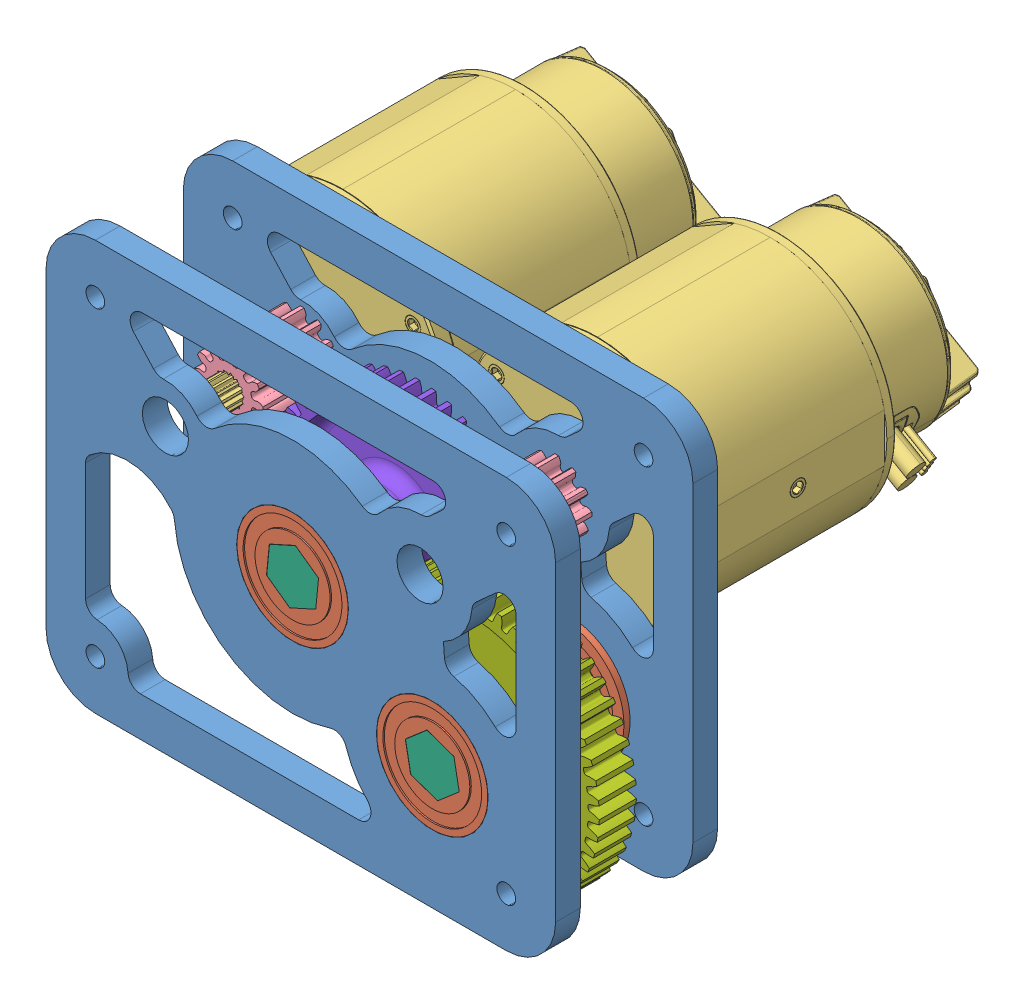
SolidWorks assembly elevator gearbox v2, configuration Default. Lengths in mm.
Overall size (142.66 117 123.61).
16 component instances, 9 part files, 32 mates.
Components (placement in the parent):
- Gearbox plate v2-1: Gearbox plate v2 [Default] at (35.2329 53.5988 97.8908) size (131.06 105.41 6.35)
- Vexpro - .5in hex bearing flanged - 217-3875-2: Vexpro - .5in hex bearing flanged - 217-3875 [Default] at (71.1722 29.5266 97.8908) x (-0.757843 -0.652437 0) z (-0.652437 0.757843 0) size (31.12 7.94 31.12)
- Vexpro - .5in hex bearing flanged - 217-3875-3: Vexpro - .5in hex bearing flanged - 217-3875 [Default] at (35.2329 53.5988 97.8908) x (0.036345 -0.999339 0) z (-0.999339 -0.036345 0) size (31.12 7.94 31.12)
- Vexpro - Falcon 500 - 217-6515-1: Vexpro - Falcon 500 - 217-6515 [Default] at (66.7919 64.2976 60.9528) size (60.01 60.01 116.76)
- Vexpro - Falcon 500 - 217-6515-2: Vexpro - Falcon 500 - 217-6515 [Default] at (1.3077 64.4878 60.9528) size (60.01 60.01 116.76)
- WCP 12t pinion gear-1: WCP 12t pinion gear [Default] at (2.5403 70.7236 113.7658) x (0.857821 0.513949 0) z (0 0 1) size (17.78 17.78 19.05)
- WCP 12t pinion gear-2: WCP 12t pinion gear [Default] at (68.0245 70.5334 113.7658) x (0.857821 0.513949 0) z (0 0 1) size (17.78 17.78 19.05)
- Gearbox plate v2-2: Gearbox plate v2 [Default] at (35.2329 53.5988 133.2032) size (131.06 105.41 6.35)
- Vexpro - .5in hex bearing flanged - 217-3875-4: Vexpro - .5in hex bearing flanged - 217-3875 [Default] at (35.2329 53.5988 139.5532) x (-0.812177 0.583411 0) z (-0.583411 -0.812177 0) size (31.12 7.94 31.12)
- Vexpro - .5in hex bearing flanged - 217-3875-5: Vexpro - .5in hex bearing flanged - 217-3875 [Default] at (71.1722 29.5266 139.5532) x (0.943998 -0.329951 0) z (0.329951 0.943998 0) size (31.12 7.94 31.12)
- 18t gear wcp-1: 18t gear wcp [Default] at (35.2329 53.5988 124.8021) x (-1 0 0) z (0 0 1) size (25.17 25.4 12.65)
- 1.871 in shaft-1: 1.871 in shaft [Default] at (35.2542 53.5835 -317.6468) x (0.911337 0.411661 0) z (0 0 1) size (14.48 12.67 47.52)
- 50t Pocketed 20DP Gear WCP-0119-1: 50t Pocketed 20DP Gear WCP-0119 [Default] at (71.1722 29.5266 124.8529) x (-0.919303 -0.39355 0) z (0 0 -1) size (65.97 66.04 12.65)
- 42t Pocketed 20DP Gear WCP-0117-1: 42t Pocketed 20DP Gear WCP-0117 [Default] at (35.2329 53.5988 112.1529) size (55.8 55.88 12.65)
- 1.871 in shaft-2: 1.871 in shaft [Default] at (71.1969 29.5179 -317.6468) x (0.757745 0.65255 0) z (0 0 1) size (14.48 12.67 47.52)
- Vexpro - .5in acetal hex spacer - 217 - 3261-1: Vexpro - .5in acetal hex spacer - 217 - 3261 [Default] at (71.1722 29.5266 112.1783) size (19.5 19.5 12.7)
Mates (geometry in assembly coordinates):
- Concentric3: concentric anti-aligned: cylinder of Gearbox plate v2-1 through (71.1722 29.5266 104.2408) axis (0 0 -1) radius 14.3891; cylinder of Vexpro - .5in hex bearing flanged - 217-3875-2 through (71.1722 29.5266 97.8908) axis (0 0 1) radius 14.2748
- Concentric4: concentric anti-aligned: cylinder of Gearbox plate v2-1 through (35.2329 53.5988 104.2408) axis (0 0 -1) radius 14.3891; cylinder of Vexpro - .5in hex bearing flanged - 217-3875-3 through (35.2329 53.5988 97.8908) axis (0 0 1) radius 14.2748
- Coincident5: coincident anti-aligned: plane of Gearbox plate v2-1 through (35.2329 53.5988 104.2408) normal (0 0 1); plane of Vexpro - .5in hex bearing flanged - 217-3875-3 through (35.7984 38.0516 104.2408) normal (0 0 -1)
- Coincident6: coincident anti-aligned: plane of Gearbox plate v2-1 through (35.2329 53.5988 104.2408) normal (0 0 1); plane of Vexpro - .5in hex bearing flanged - 217-3875-2 through (59.382 19.3763 104.2408) normal (0 0 -1)
- Coincident7: coincident anti-aligned: plane of Gearbox plate v2-1 through (35.2329 53.5988 97.8908) normal (0 0 -1); plane of Vexpro - Falcon 500 - 217-6515-1 through (63.262 62.2845 97.8908) normal (0 0 1)
- Coincident8: coincident anti-aligned: plane of Gearbox plate v2-1 through (35.2329 53.5988 97.8908) normal (0 0 -1); plane of Vexpro - Falcon 500 - 217-6515-2 through (-2.2222 62.4748 97.8908) normal (0 0 1)
- Concentric7: concentric aligned: circle of Vexpro - Falcon 500 - 217-6515-2; circle of WCP 12t pinion gear-1
- Coincident9: coincident anti-aligned: plane of Gearbox plate v2-1 through (35.2329 53.5988 104.2408) normal (0 0 1); plane of WCP 12t pinion gear-1 through (2.5403 70.7236 104.2408) normal (0 0 -1)
- Coincident10: coincident anti-aligned: plane of Gearbox plate v2-1 through (35.2329 53.5988 104.2408) normal (0 0 1); plane of WCP 12t pinion gear-2 through (68.0245 70.5334 104.2408) normal (0 0 -1)
- Concentric8: concentric aligned: circle of Vexpro - Falcon 500 - 217-6515-1; circle of WCP 12t pinion gear-2
- Coincident37: coincident aligned: plane of Gearbox plate v2-1 through (102.8961 53.5988 104.2408) normal (1 0 0); plane of Gearbox plate v2-2 through (102.8961 53.5988 139.5532) normal (1 0 0)
- Coincident38: coincident aligned: plane of Gearbox plate v2-1 through (35.2329 103.1866 104.2408) normal (0 1 0); plane of Gearbox plate v2-2 through (35.2329 103.1866 139.5532) normal (0 1 0)
- Concentric19: concentric aligned: cylinder of Gearbox plate v2-2 through (35.2329 53.5988 139.5532) axis (0 0 -1) radius 14.3891; cylinder of Vexpro - .5in hex bearing flanged - 217-3875-4 through (35.2329 53.5988 139.5532) axis (0 0 -1) radius 14.2748
- Coincident39: coincident anti-aligned: plane of Gearbox plate v2-2 through (35.2329 53.5988 133.2032) normal (0 0 -1); plane of Vexpro - .5in hex bearing flanged - 217-3875-4 through (22.5975 62.6752 133.2032) normal (0 0 1)
- Coincident40: coincident anti-aligned: plane of Gearbox plate v2-2 through (35.2329 53.5988 133.2032) normal (0 0 -1); plane of Vexpro - .5in hex bearing flanged - 217-3875-5 through (85.8584 24.3933 133.2032) normal (0 0 1)
- Concentric20: concentric anti-aligned: circle of Gearbox plate v2-2; circle of Vexpro - .5in hex bearing flanged - 217-3875-5
- Coincident46: coincident aligned: plane of Vexpro - .5in hex bearing flanged - 217-3875-4 through (27.3938 59.2299 139.5532) normal (0 0 1); plane of 1.871 in shaft-1 through (41.9231 56.5959 139.5532) normal (0 0 1)
- Coincident47: coincident anti-aligned: plane of Vexpro - .5in hex bearing flanged - 217-3875-4 through (41.9257 56.622 139.5532) normal (-0.995072 0.09916 0); plane of 1.871 in shaft-1 through (41.1975 49.3143 139.5532) normal (0.995072 -0.09916 0)
- Coincident48: coincident anti-aligned: line of Vexpro - .5in hex bearing flanged - 217-3875-4 through (41.1975 49.3143 139.5532) axis (-0.911337 -0.411661 0); line of 1.871 in shaft-1 through (34.7959 46.4226 139.5532) axis (0.911337 0.411661 0)
- Coincident49: coincident anti-aligned: plane of Vexpro - .5in hex bearing flanged - 217-3875-3 through (35.4637 47.253 105.8283) normal (0 0 1); plane of 42t Pocketed 20DP Gear WCP-0117-1 through (35.2329 53.5988 105.8283) normal (0 0 -1)
- Concentric21: concentric aligned: circle of Vexpro - .5in hex bearing flanged - 217-3875-4; circle of 42t Pocketed 20DP Gear WCP-0117-1
- Coincident50: coincident anti-aligned: plane of 18t gear wcp-1 through (35.2329 53.5988 118.4775) normal (0 0 -1); plane of 42t Pocketed 20DP Gear WCP-0117-1 through (35.2329 53.5988 118.4775) normal (0 0 1)
- Concentric22: concentric anti-aligned: circle of 18t gear wcp-1; circle of 42t Pocketed 20DP Gear WCP-0117-1
- Concentric23: concentric anti-aligned: circle of Vexpro - .5in hex bearing flanged - 217-3875-5; circle of 50t Pocketed 20DP Gear WCP-0119-1
- Coincident60: coincident aligned: plane of Vexpro - .5in hex bearing flanged - 217-3875-5 through (80.2836 26.3419 139.5532) normal (0 0 1); plane of 1.871 in shaft-2 through (76.7418 34.2931 139.5532) normal (0 0 1)
- Coincident61: coincident anti-aligned: line of Vexpro - .5in hex bearing flanged - 217-3875-5 through (76.737 34.3188 139.5532) axis (0.186253 -0.982502 0); line of 1.871 in shaft-2 through (78.0502 27.3916 139.5532) axis (-0.186253 0.982502 0)
- Coincident62: coincident anti-aligned: line of Vexpro - .5in hex bearing flanged - 217-3875-5 through (78.1048 27.1034 139.5532) axis (-0.757745 -0.65255 0); line of 1.871 in shaft-2 through (72.7821 22.5197 139.5532) axis (0.757745 0.65255 0)
- Concentric25: concentric anti-aligned: cylinder of Gearbox plate v2-1 through (68.0245 70.5334 104.2408) axis (0 0 -1) radius 5.9309; cone of Vexpro - Falcon 500 - 217-6515-1 through (68.0245 70.5334 97.8908) axis (0 0 1)
- Concentric26: concentric anti-aligned: cylinder of Gearbox plate v2-1 through (2.5403 70.7236 104.2408) axis (0 0 -1) radius 5.9309; cone of Vexpro - Falcon 500 - 217-6515-2 through (2.5403 70.7236 97.8908) axis (0 0 1)
- Coincident63: coincident anti-aligned: plane of Vexpro - .5in hex bearing flanged - 217-3875-2 through (66.3599 25.3836 105.8283) normal (0 0 1); plane of Vexpro - .5in acetal hex spacer - 217 - 3261-1 through (71.1722 29.5266 105.8283) normal (0 0 -1)
- Concentric27: concentric anti-aligned: cylinder of Vexpro - .5in hex bearing flanged - 217-3875-2 through (71.1722 29.5266 97.8908) axis (0 0 1) radius 15.5575; cylinder of Vexpro - .5in acetal hex spacer - 217 - 3261-1 through (71.1722 29.5266 118.5283) axis (0 0 -1) radius 9.75
- Coincident64: coincident anti-aligned: plane of 50t Pocketed 20DP Gear WCP-0119-1 through (71.1722 29.5266 118.5283) normal (0 0 -1); plane of Vexpro - .5in acetal hex spacer - 217 - 3261-1 through (71.1722 29.5266 118.5283) normal (0 0 1)
